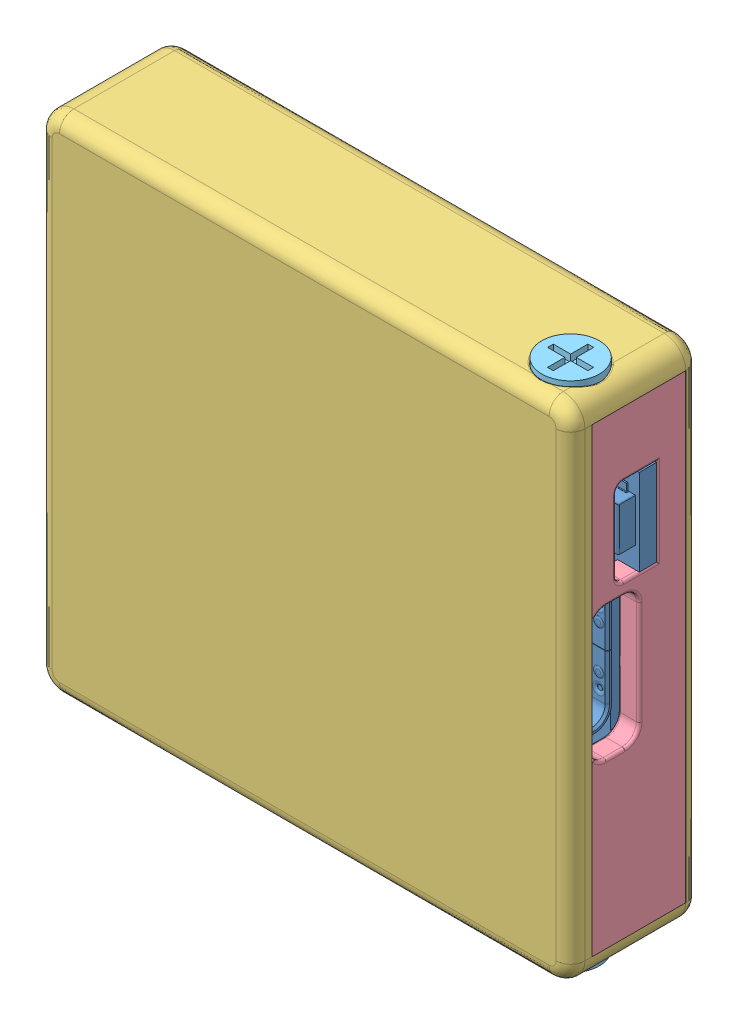
SolidWorks assembly 装配体1, configuration 默认. Lengths in mm.
Overall size (37.02 35.6 10.07).
6 component instances, 5 part files, 13 mates.
Components (placement in the parent):
- 8266电脑数据显示-1: 8266电脑数据显示 [默认] at (-21.1371 0.1446 34.1357) size (35.5 31.5 8.96)
- 1.54tft屏幕-1: 1.54tft屏幕 [默认] at (-4.2771 0.1446 32.9357) x (0 -1 0) z (1 0 0) size (31.52 2.03 33.72)
- 外壳-1: 外壳 [默认] at (14.3629 0.1446 38.9057) x (0 -1 0) z (0 0 -1) size (35.06 37 9)
- 内壳-1: 内壳 [默认] at (14.3629 0.1446 37.4357) x (0 -1 0) z (0 0 -1) size (32 35.52 6.5)
- M2_2.5-1: M2_2.5 [默认] at (11.3629 17.9446 35.9057) size (4 3.4 4)
- M2_2.5-2: M2_2.5 [默认] at (11.3629 -17.6554 35.9057) x (-0.993178 0 -0.116611) z (-0.116611 0 0.993178) size (4 3.4 4)
Mates (geometry in assembly coordinates):
- 距离2: distance = 0.25 mm anti-aligned: plane of 8266电脑数据显示-1 through (12.6129 -15.6054 32.9357) normal (0 -1 0); plane of 外壳-1 through (-21.5371 -15.8554 37.4057) normal (0 1 0)
- 重合5: coincident anti-aligned: plane of 8266电脑数据显示-1 through (-21.1371 -15.3554 32.9357) normal (0 0 -1); plane of 1.54tft屏幕-1 through (-4.2771 0.1446 32.9357) normal (0 0 1)
- 重合6: coincident aligned: plane of 8266电脑数据显示-1 through (-21.1371 -15.3554 32.9357) normal (-1 0 0); plane of 1.54tft屏幕-1 through (-21.1371 15.9046 31.0357) normal (-1 0 0)
- 距离3: distance = 0.01 mm aligned: plane of 8266电脑数据显示-1 through (12.6129 -15.6054 32.9357) normal (0 -1 0); plane of 1.54tft屏幕-1 through (12.5829 -15.6154 31.0357) normal (0 -1 0)
- 重合8: coincident anti-aligned: plane of 1.54tft屏幕-1 through (-4.2771 0.1446 30.9057) normal (0 0 -1); plane of 外壳-1 through (-21.5371 -15.8554 30.9057) normal (0 0 1)
- 重合10: coincident anti-aligned: plane of 8266电脑数据显示-1 through (12.8629 15.6446 32.9357) normal (1 0 0); plane of 内壳-1 through (12.8629 16.1446 34.2357) normal (-1 0 0)
- 距离5: distance = 0.25 mm aligned: plane of 8266电脑数据显示-1 through (12.6129 -15.6054 32.9357) normal (0 -1 0); plane of 内壳-1 through (14.3629 -15.8554 30.9357) normal (0 -1 0)
- 重合11: coincident anti-aligned: plane of 8266电脑数据显示-1 through (-21.1371 -15.3554 32.9357) normal (0 0 -1); plane of 内壳-1 through (12.1629 11.6446 32.9357) normal (0 0 1)
- 重合12: coincident: line of 外壳-1 through (14.3629 -15.8554 37.4057) axis (0 0 -1); plane of 内壳-1 through (14.3629 0.1446 30.9357) normal (1 0 0)
- 同心1: concentric anti-aligned: cylinder of 外壳-1 through (11.3629 -17.3554 35.9057) axis (0 1 0) radius 0.9; cylinder of M2_2.5-1 through (11.3629 14.6446 35.9057) axis (0 -1 0) radius 2
- 重合14: coincident anti-aligned: plane of 外壳-1 through (11.3629 17.1446 35.9057) normal (0 1 0); plane of M2_2.5-1 through (13.3629 17.1446 35.9057) normal (0 -1 0)
- 同心2: concentric aligned: cylinder of 外壳-1 through (11.3629 -17.3554 35.9057) axis (0 1 0) radius 0.9; cylinder of M2_2.5-2 through (11.3629 -14.3554 35.9057) axis (0 1 0) radius 2
- 重合15: coincident anti-aligned: plane of 外壳-1 through (11.3629 -16.8554 35.9057) normal (0 -1 0); plane of M2_2.5-2 through (9.3765 -16.8554 35.6725) normal (0 1 0)
